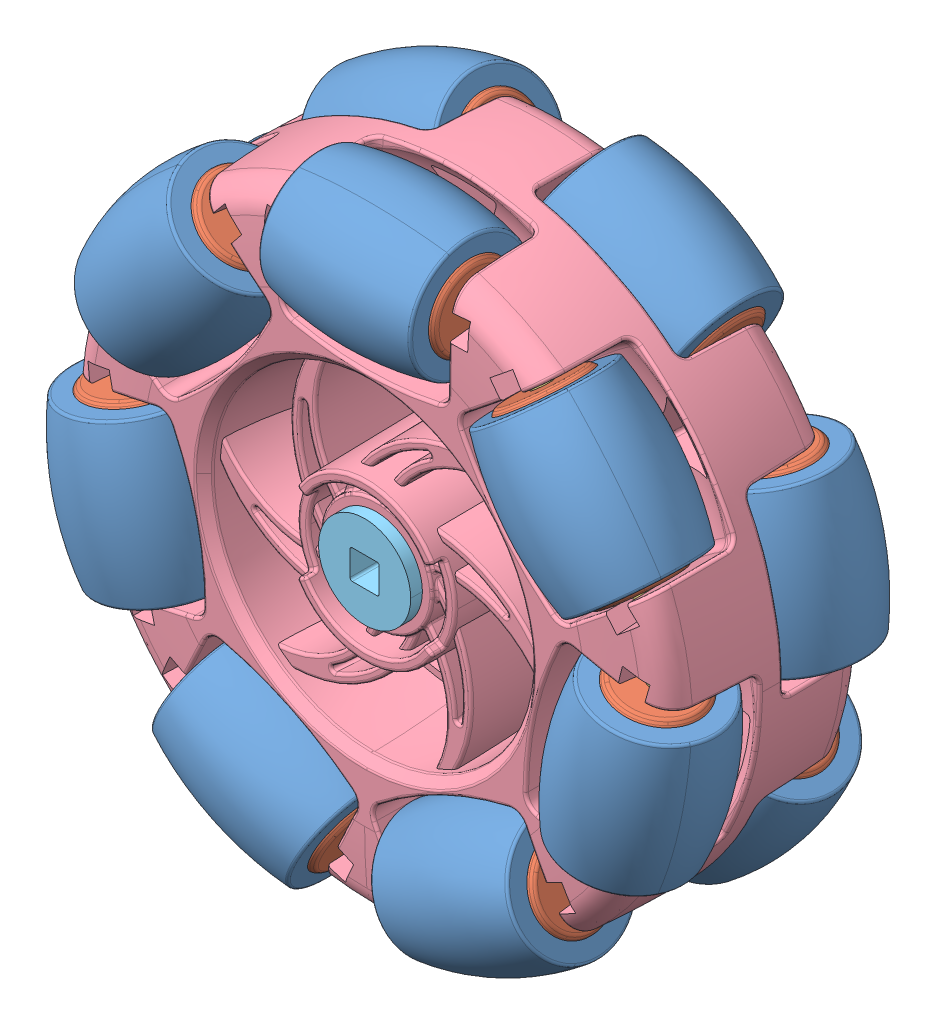
SolidWorks assembly 2.75 Omni with inserts (276-1902) , configuration Default. Lengths in mm.
Overall size (87.15 87.98 47.75).
61 component instances, 5 part files, 6 mates.
Components (placement in the parent):
- 2.75 Omni-Directional Wheel - Double Roller (276-1902) -1: 2.75 Omni-Directional Wheel - Double Roller (276-1902)  [Default] at (25.8037 49.8406 68.5807) size (87.15 87.98 47.75)
  - 2.75 Omni-Directional Wheel - Double Roller (276-1902) .step-1: 2.75 Omni-Directional Wheel - Double Roller (276-1902) .step [Default] at origin size (87.15 87.98 47.75)
    - 276-1902-010 Rev1.step-1: 276-1902-010 Rev1.step [Default] at (0 27.5 8) x (1 0 0) z (0 0.828233 0.560383) size (23 27.81 20.35)
      - 276-1902-011 Rev1.step-1: 276-1902-011 Rev1.step [Default] at (0 -6.325 -26.7627) x (1 0 0) z (0 -0.973191 0.23) size (16.5 15 25.03)
      - 276-1902-012 Rev1.step-1: 276-1902-012 Rev1.step [Default] at origin size (17.5 10.34 18.34)
      - 276-1902-003 Rev1.step-1: 276-1902-003 Rev1.step [Default] x (0 -0.928523 0.371275) z (1 0 0) size (2 2 23)
    - 276-1902-010 Rev1.step-2: 276-1902-010 Rev1.step [Default] at (0 -27.5 -8) x (1 0 0) z (0 0.410464 0.911877) size (23 27.81 20.35)
      - 276-1902-011 Rev1.step-1: 276-1902-011 Rev1.step [Default] at (0 -6.325 -26.7627) x (1 0 0) z (0 -0.973191 0.23) size (16.5 15 25.03)
      - 276-1902-012 Rev1.step-1: 276-1902-012 Rev1.step [Default] at origin size (17.5 10.34 18.34)
      - 276-1902-003 Rev1.step-1: 276-1902-003 Rev1.step [Default] x (0 -0.928523 0.371275) z (1 0 0) size (2 2 23)
    - 276-1902-010 Rev1.step-3: 276-1902-010 Rev1.step [Default] at (-21.5004 -17.146 -8) x (0.62349 -0.781831 0) z (0.320913 0.25592 0.911877) size (23 27.81 20.35)
      - 276-1902-011 Rev1.step-1: 276-1902-011 Rev1.step [Default] at (0 -6.325 -26.7627) x (1 0 0) z (0 -0.973191 0.23) size (16.5 15 25.03)
      - 276-1902-012 Rev1.step-1: 276-1902-012 Rev1.step [Default] at origin size (17.5 10.34 18.34)
      - 276-1902-003 Rev1.step-1: 276-1902-003 Rev1.step [Default] x (0 -0.928523 0.371275) z (1 0 0) size (2 2 23)
    - 276-1902-010 Rev1.step-4: 276-1902-010 Rev1.step [Default] at (-26.8105 6.1193 -8) x (-0.222521 -0.974928 0) z (0.400172 -0.091337 0.911877) size (23 27.81 20.35)
      - 276-1902-011 Rev1.step-1: 276-1902-011 Rev1.step [Default] at (0 -6.325 -26.7627) x (1 0 0) z (0 -0.973191 0.23) size (16.5 15 25.03)
      - 276-1902-012 Rev1.step-1: 276-1902-012 Rev1.step [Default] at origin size (17.5 10.34 18.34)
      - 276-1902-003 Rev1.step-1: 276-1902-003 Rev1.step [Default] x (0 -0.928523 0.371275) z (1 0 0) size (2 2 23)
    - 276-1902-010 Rev1.step-5: 276-1902-010 Rev1.step [Default] at (-11.9318 24.7766 -8) x (-0.900969 -0.433884 0) z (0.178093 -0.369815 0.911877) size (23 27.81 20.35)
      - 276-1902-011 Rev1.step-1: 276-1902-011 Rev1.step [Default] at (0 -6.325 -26.7627) x (1 0 0) z (0 -0.973191 0.23) size (16.5 15 25.03)
      - 276-1902-012 Rev1.step-1: 276-1902-012 Rev1.step [Default] at origin size (17.5 10.34 18.34)
      - 276-1902-003 Rev1.step-1: 276-1902-003 Rev1.step [Default] x (0 -0.928523 0.371275) z (1 0 0) size (2 2 23)
    - 276-1902-010 Rev1.step-6: 276-1902-010 Rev1.step [Default] at (11.9318 24.7766 -8) x (-0.900969 0.433884 0) z (-0.178093 -0.369815 0.911877) size (23 27.81 20.35)
      - 276-1902-011 Rev1.step-1: 276-1902-011 Rev1.step [Default] at (0 -6.325 -26.7627) x (1 0 0) z (0 -0.973191 0.23) size (16.5 15 25.03)
      - 276-1902-012 Rev1.step-1: 276-1902-012 Rev1.step [Default] at origin size (17.5 10.34 18.34)
      - 276-1902-003 Rev1.step-1: 276-1902-003 Rev1.step [Default] x (0 -0.928523 0.371275) z (1 0 0) size (2 2 23)
    - 276-1902-010 Rev1.step-7: 276-1902-010 Rev1.step [Default] at (26.8105 6.1193 -8) x (-0.222521 0.974928 0) z (-0.400172 -0.091337 0.911877) size (23 27.81 20.35)
      - 276-1902-011 Rev1.step-1: 276-1902-011 Rev1.step [Default] at (0 -6.325 -26.7627) x (1 0 0) z (0 -0.973191 0.23) size (16.5 15 25.03)
      - 276-1902-012 Rev1.step-1: 276-1902-012 Rev1.step [Default] at origin size (17.5 10.34 18.34)
      - 276-1902-003 Rev1.step-1: 276-1902-003 Rev1.step [Default] x (0 -0.928523 0.371275) z (1 0 0) size (2 2 23)
    - 276-1902-010 Rev1.step-8: 276-1902-010 Rev1.step [Default] at (21.5004 -17.146 -8) x (0.62349 0.781831 0) z (-0.320913 0.25592 0.911877) size (23 27.81 20.35)
      - 276-1902-011 Rev1.step-1: 276-1902-011 Rev1.step [Default] at (0 -6.325 -26.7627) x (1 0 0) z (0 -0.973191 0.23) size (16.5 15 25.03)
      - 276-1902-012 Rev1.step-1: 276-1902-012 Rev1.step [Default] at origin size (17.5 10.34 18.34)
      - 276-1902-003 Rev1.step-1: 276-1902-003 Rev1.step [Default] x (0 -0.928523 0.371275) z (1 0 0) size (2 2 23)
    - 276-1902-010 Rev1.step-9: 276-1902-010 Rev1.step [Default] at (21.5004 17.146 8) x (0.62349 -0.781831 0) z (0.647539 0.516395 0.560383) size (23 27.81 20.35)
      - 276-1902-011 Rev1.step-1: 276-1902-011 Rev1.step [Default] at (0 -6.325 -26.7627) x (1 0 0) z (0 -0.973191 0.23) size (16.5 15 25.03)
      - 276-1902-012 Rev1.step-1: 276-1902-012 Rev1.step [Default] at origin size (17.5 10.34 18.34)
      - 276-1902-003 Rev1.step-1: 276-1902-003 Rev1.step [Default] x (0 -0.928523 0.371275) z (1 0 0) size (2 2 23)
    - 276-1902-010 Rev1.step-10: 276-1902-010 Rev1.step [Default] at (26.8105 -6.1193 8) x (-0.222521 -0.974928 0) z (0.807468 -0.184299 0.560383) size (23 27.81 20.35)
      - 276-1902-011 Rev1.step-1: 276-1902-011 Rev1.step [Default] at (0 -6.325 -26.7627) x (1 0 0) z (0 -0.973191 0.23) size (16.5 15 25.03)
      - 276-1902-012 Rev1.step-1: 276-1902-012 Rev1.step [Default] at origin size (17.5 10.34 18.34)
      - 276-1902-003 Rev1.step-1: 276-1902-003 Rev1.step [Default] x (0 -0.928523 0.371275) z (1 0 0) size (2 2 23)
    - 276-1902-010 Rev1.step-11: 276-1902-010 Rev1.step [Default] at (11.9318 -24.7766 8) x (-0.900969 -0.433884 0) z (0.359357 -0.746212 0.560383) size (23 27.81 20.35)
      - 276-1902-011 Rev1.step-1: 276-1902-011 Rev1.step [Default] at (0 -6.325 -26.7627) x (1 0 0) z (0 -0.973191 0.23) size (16.5 15 25.03)
      - 276-1902-012 Rev1.step-1: 276-1902-012 Rev1.step [Default] at origin size (17.5 10.34 18.34)
      - 276-1902-003 Rev1.step-1: 276-1902-003 Rev1.step [Default] x (0 -0.928523 0.371275) z (1 0 0) size (2 2 23)
    - 276-1902-010 Rev1.step-12: 276-1902-010 Rev1.step [Default] at (-11.9318 -24.7766 8) x (-0.900969 0.433884 0) z (-0.359357 -0.746212 0.560383) size (23 27.81 20.35)
      - 276-1902-011 Rev1.step-1: 276-1902-011 Rev1.step [Default] at (0 -6.325 -26.7627) x (1 0 0) z (0 -0.973191 0.23) size (16.5 15 25.03)
      - 276-1902-012 Rev1.step-1: 276-1902-012 Rev1.step [Default] at origin size (17.5 10.34 18.34)
      - 276-1902-003 Rev1.step-1: 276-1902-003 Rev1.step [Default] x (0 -0.928523 0.371275) z (1 0 0) size (2 2 23)
    - 276-1902-010 Rev1.step-13: 276-1902-010 Rev1.step [Default] at (-26.8105 -6.1193 8) x (-0.222521 0.974928 0) z (-0.807468 -0.184299 0.560383) size (23 27.81 20.35)
      - 276-1902-011 Rev1.step-1: 276-1902-011 Rev1.step [Default] at (0 -6.325 -26.7627) x (1 0 0) z (0 -0.973191 0.23) size (16.5 15 25.03)
      - 276-1902-012 Rev1.step-1: 276-1902-012 Rev1.step [Default] at origin size (17.5 10.34 18.34)
      - 276-1902-003 Rev1.step-1: 276-1902-003 Rev1.step [Default] x (0 -0.928523 0.371275) z (1 0 0) size (2 2 23)
    - 276-1902-010 Rev1.step-14: 276-1902-010 Rev1.step [Default] at (-21.5004 17.146 8) x (0.62349 0.781831 0) z (-0.647539 0.516395 0.560383) size (23 27.81 20.35)
      - 276-1902-011 Rev1.step-1: 276-1902-011 Rev1.step [Default] at (0 -6.325 -26.7627) x (1 0 0) z (0 -0.973191 0.23) size (16.5 15 25.03)
      - 276-1902-012 Rev1.step-1: 276-1902-012 Rev1.step [Default] at origin size (17.5 10.34 18.34)
      - 276-1902-003 Rev1.step-1: 276-1902-003 Rev1.step [Default] x (0 -0.928523 0.371275) z (1 0 0) size (2 2 23)
    - 276-1902-002 Rev3.step-1: 276-1902-002 Rev3.step [Default] at origin size (66.55 66.02 25.07)
- Metal Shaft Inserts (276-3881-002)-1: Metal Shaft Inserts (276-3881-002) [Default] at (25.8037 49.8406 79.8307) x (0 -1 0) z (1 0 0) size (10.03 5.08 10.03)
- Metal Shaft Inserts (276-3881-002)-2: Metal Shaft Inserts (276-3881-002) [Default] at (25.8037 49.8406 57.3307) x (1 0 0) z (0 -1 0) size (10.03 5.08 10.03)
Mates (geometry in assembly coordinates):
- Concentric1: concentric anti-aligned: circle of 2.75 Omni-Directional Wheel - Double Roller (276-1902) -1/2.75 Omni-Directional Wheel - Double Roller (276-1902) .step-1/276-1902-002 Rev3.step-1; circle of Metal Shaft Inserts (276-3881-002)-1
- Parallel1: parallel aligned: plane of 2.75 Omni-Directional Wheel - Double Roller (276-1902) -1/2.75 Omni-Directional Wheel - Double Roller (276-1902) .step-1/276-1902-002 Rev3.step-1 through (22.6287 46.6656 79.8362) normal (1 0 0); plane of Metal Shaft Inserts (276-3881-002)-1 through (28.9533 52.9902 74.7507) normal (1 0 0)
- Coincident2: coincident anti-aligned: plane of 2.75 Omni-Directional Wheel - Double Roller (276-1902) -1/2.75 Omni-Directional Wheel - Double Roller (276-1902) .step-1/276-1902-002 Rev3.step-1 through (25.8037 49.8406 78.5607) normal (0 0 1); plane of Metal Shaft Inserts (276-3881-002)-1 through (25.8037 49.8406 78.5607) normal (0 0 -1)
- Parallel2: parallel anti-aligned: plane of 2.75 Omni-Directional Wheel - Double Roller (276-1902) -1/2.75 Omni-Directional Wheel - Double Roller (276-1902) .step-1/276-1902-002 Rev3.step-1 through (28.9787 46.6656 79.8362) normal (0 1 0); plane of Metal Shaft Inserts (276-3881-002)-2 through (22.6541 46.691 62.4107) normal (0 -1 0)
- Coincident4: coincident anti-aligned: plane of 2.75 Omni-Directional Wheel - Double Roller (276-1902) -1/2.75 Omni-Directional Wheel - Double Roller (276-1902) .step-1/276-1902-002 Rev3.step-1 through (25.8037 49.8406 58.6007) normal (0 0 -1); plane of Metal Shaft Inserts (276-3881-002)-2 through (25.8037 49.8406 58.6007) normal (0 0 1)
- Concentric3: concentric aligned: circle of 2.75 Omni-Directional Wheel - Double Roller (276-1902) -1/2.75 Omni-Directional Wheel - Double Roller (276-1902) .step-1/276-1902-002 Rev3.step-1; circle of Metal Shaft Inserts (276-3881-002)-2
